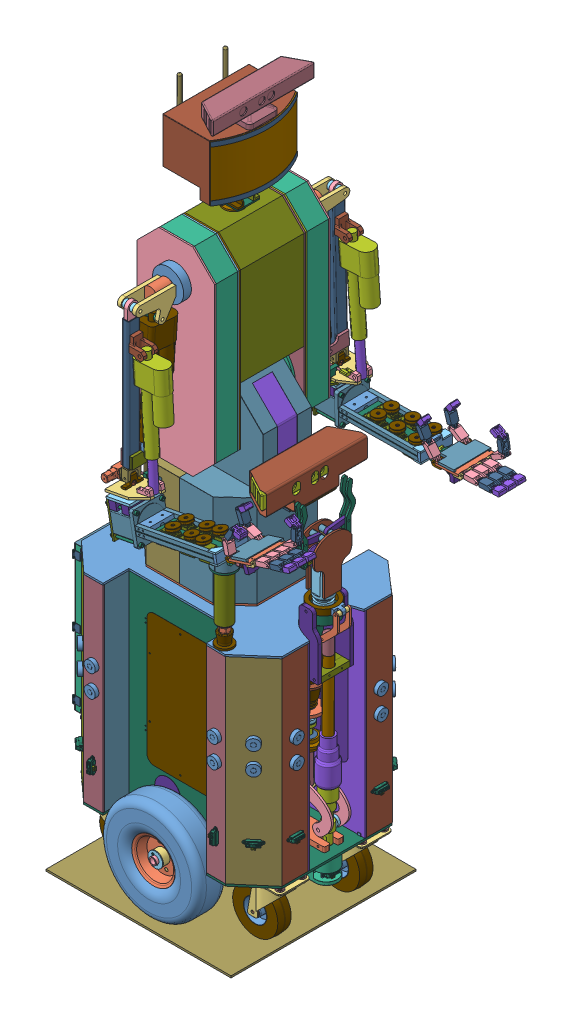
SolidWorks assembly sorbot, configuration По умолчанию. Lengths in mm. (continued)
Mates (geometry in assembly coordinates): (continued)
- Concentric42: concentric anti-aligned: cylinder of wall11-1 through (-271.9003 171.4368 -274.4564) axis (-1 0 0) radius 2; cylinder of computer.box.screw.fixture-4 through (-267.4772 171.4368 -274.4564) axis (1 0 0) radius 2
- Concentric43: concentric anti-aligned: cylinder of wall11-1 through (-271.9003 171.4368 0.207) axis (-1 0 0) radius 2; cylinder of computer.box.screw.fixture-3 through (-269.9003 171.4368 0.207) axis (1 0 0) radius 2
- Concentric44: concentric anti-aligned: cylinder of wall11-1 through (-271.9003 548.1505 0.207) axis (-1 0 0) radius 2; cylinder of computer.box.screw.fixture-2 through (-267.4772 548.1505 0.207) axis (1 0 0) radius 2
- Concentric45: concentric anti-aligned: cylinder of wall11-1 through (-271.9003 548.1505 -274.4564) axis (-1 0 0) radius 2; cylinder of computer.box.screw.fixture-1 through (-269.9003 548.1505 -274.4564) axis (1 0 0) radius 2
- Parallel10: parallel anti-aligned: plane of wall11-1 through (-271.9003 882.565 10.1667) normal (1 0 0); plane of us_sesnor_board-1 through (-254.9003 553.7811 -265.7072) normal (-1 0 0)
- Parallel11: parallel anti-aligned: plane of wall11-1 through (-271.9003 882.565 10.1667) normal (1 0 0); plane of us_sesnor_board-2 through (-254.9003 552.2966 -6.9008) normal (-1 0 0)
- Lock52: lock: unknown of wall11-1; unknown of wall-fixture-v2-1-2
- Lock54: lock: unknown of wall-fixture-v2-1-2; unknown of computer.box.screw.fixture-1
- Coincident100: coincident anti-aligned: plane of wall11-1 through (-271.9003 882.565 10.1667) normal (1 0 0); plane of wall-fixture-v2-1-1 through (-271.9003 624.2006 -10.7109) normal (-1 0 0)
- Lock55: lock: unknown of wall11-1; unknown of wall-fixture-v2-1-1
- Lock56: lock: unknown of wall-fixture-v2-1-1; unknown of computer.box.screw.fixture-2
- Coincident101: coincident: plane of us_sesnor_board-1 through (-261.9003 646.0902 -16.9266) normal (-1 0 0); plane of pillar.15mm-1 through (-261.9003 620.2581 -29.4638) normal (1 0 0)
- Coincident102: coincident: plane of us_sesnor_board-1 through (-261.9003 646.0902 -16.9266) normal (-1 0 0); plane of pillar.15mm-2 through (-261.9003 672.3698 -3.6565) normal (1 0 0)
- Coincident103: coincident: plane of us_sesnor_board-2 through (-278.4971 649.7829 -78.0769) normal (-1 0 0); plane of pillar.15mm-3 through (-278.4971 623.9508 -90.6141) normal (1 0 0)
- Coincident104: coincident: plane of us_sesnor_board-2 through (-278.4971 649.7829 -78.0769) normal (-1 0 0); plane of pillar.15mm-4 through (-278.4971 676.0625 -64.8068) normal (1 0 0)
- Concentric46: concentric anti-aligned: cylinder of us_sesnor_board-2 through (-278.4971 623.9508 -90.6141) axis (1 0 0) radius 1.5; cylinder of pillar.15mm-3 through (-278.4971 623.9508 -90.6141) axis (-1 0 0) radius 1.5
- Concentric47: concentric anti-aligned: cylinder of us_sesnor_board-2 through (-278.4971 676.0625 -64.8068) axis (1 0 0) radius 1.5; cylinder of pillar.15mm-4 through (-278.4971 676.0625 -64.8068) axis (-1 0 0) radius 1.5
- Concentric48: concentric anti-aligned: cylinder of us_sesnor_board-1 through (-261.9003 672.3698 -3.6565) axis (1 0 0) radius 1.5; cylinder of pillar.15mm-2 through (-261.9003 672.3698 -3.6565) axis (-1 0 0) radius 1.5
- Concentric49: concentric anti-aligned: cylinder of us_sesnor_board-1 through (-261.9003 620.2581 -29.4638) axis (1 0 0) radius 1.5; cylinder of pillar.15mm-1 through (-261.9003 620.2581 -29.4638) axis (-1 0 0) radius 1.5
- Lock57: lock: unknown of us_sesnor_board-2; unknown of pillar.15mm-3
- Lock58: lock: unknown of us_sesnor_board-2; unknown of pillar.15mm-4
- Lock59: lock: unknown of us_sesnor_board-1; unknown of pillar.15mm-1
- Lock60: lock: unknown of us_sesnor_board-1; unknown of pillar.15mm-2
- Coincident106: coincident anti-aligned: plane of wall-fixture-v2-1-2 through (-269.9003 624.1077 -280.8026) normal (1 0 0); plane of pillar.15mm-1 through (-269.9003 527.949 -278.2445) normal (-1 0 0)
- Coincident108: coincident anti-aligned: plane of wall-fixture-v2-1-1 through (-269.9003 624.2006 -10.7109) normal (1 0 0); plane of pillar.15mm-4 through (-269.9003 578.5762 6.3693) normal (-1 0 0)
- Coincident111: coincident: unknown of us_sesnor_board-3; unknown of pillar.10mm-5
- Coincident112: coincident: unknown of us_sesnor_board-3; unknown of pillar.10mm-6
- Concentric51: concentric anti-aligned: cylinder of us_sesnor_board-3 through (-93.4926 309.8196 -440.0551) axis (0 1 0) radius 1.5; cylinder of pillar.10mm-6 through (-93.4926 309.8196 -440.0551) axis (0 -1 0) radius 1.5
- Concentric52: concentric anti-aligned: cylinder of us_sesnor_board-3 through (-145.6043 309.8196 -414.2478) axis (0 1 0) radius 1.5; cylinder of pillar.10mm-5 through (-145.6043 309.8196 -414.2478) axis (0 -1 0) radius 1.5
- Coincident113: coincident: plane of us_sesnor_board-4 through (-60.2671 262.1055 -397.1446) normal (0 -1 0); plane of pillar.10mm-8 through (-34.435 262.1055 -409.6819) normal (0 1 0)
- Coincident114: coincident: plane of us_sesnor_board-4 through (-60.2671 262.1055 -397.1446) normal (0 -1 0); plane of pillar.10mm-7 through (-86.5467 262.1055 -383.8745) normal (0 1 0)
- Concentric53: concentric aligned: cylinder of us_sesnor_board-4 through (-86.5467 262.1055 -383.8745) axis (0 1 0) radius 1.5; circle of pillar.10mm-7
- Concentric54: concentric anti-aligned: cylinder of us_sesnor_board-4 through (-34.435 262.1055 -409.6819) axis (0 1 0) radius 1.5; cylinder of pillar.10mm-8 through (-34.435 262.1055 -409.6819) axis (0 -1 0) radius 1.5
- Lock61: lock: unknown of us_sesnor_board-3; unknown of pillar.10mm-5
- Lock62: lock: unknown of us_sesnor_board-3; unknown of pillar.10mm-6
- Lock63: lock: unknown of us_sesnor_board-4; unknown of pillar.10mm-7
- Lock64: lock: unknown of us_sesnor_board-4; unknown of pillar.10mm-8
- Coincident117: coincident anti-aligned: plane of wall7-v1-2 through (-197.4428 -52.2153 -351.9628) normal (0.67421 0 0.73854); plane of pillar.10mm-5 through (-235.454 251.2596 -317.2625) normal (-0.67421 0 -0.73854)
- Coincident118: coincident anti-aligned: plane of wall7-v1-1 through (-271.8817 -52.2153 10.1837) normal (0.67421 0 -0.73854); plane of pillar.10mm-7 through (-215.1295 251.2596 61.9925) normal (-0.67421 0 0.73854)
- Lock65: lock: unknown of bottom-2; unknown of wall7-v1-2
- Lock68: lock: unknown of bottom-2; unknown of wall-fixture-v1-2
- Parallel17: parallel anti-aligned: plane of wall-fixture-v2-1 through (-212.277 624.3178 64.5573) normal (-0.73854 -0.000294 -0.67421); unknown of DC-DC-12-24-1
- Parallel18: parallel anti-aligned: plane of wall7-v1-1 through (-271.8817 -52.2153 10.1837) normal (0.67421 0 -0.73854); unknown of DC-DC-12-24-1
- Coincident119: coincident anti-aligned: plane of wall7-v1-1 through (-271.8817 -52.2153 10.1837) normal (0.67421 0 -0.73854); line of DC-DC-12-24-fixture-1 through (-218.8855 352.3898 58.5637) axis (-0.67421 0 0.73854)
- Lock69: lock: unknown of wall7-v1-1; unknown of wall-fixture-v2-1
- Parallel20: parallel aligned: plane of wall-fixture-v2-1 through (-212.277 624.3178 64.5573) normal (-0.73854 -0.000294 -0.67421); unknown of DC-DC-12-24-fixture-1
- Coincident124: coincident anti-aligned: unknown of DC-DC-12-24-1; line of DC-DC-12-24-fixture-p1-1 through (-195.7071 367.4849 54.6738) axis (0.67421 0 -0.73854)
- Coincident125: coincident anti-aligned: unknown of DC-DC-12-24-fixture-1; line of DC-DC-12-24-fixture-p2-1 through (-197.3861 337.4849 56.5261) axis (-0.67421 0 0.73854)
- Coincident126: coincident aligned: unknown of DC-DC-12-24-fixture-p2-1; unknown of DC-DC-12-24-fixture-p1-1
- Coincident127: coincident aligned: unknown of DC-DC-12-24-fixture-p1-1; unknown of DC-DC-12-24-fixture-p2-1
- Coincident128: coincident anti-aligned: line of DC-DC-12-24-fixture-p1-1 through (-197.0555 367.4849 56.1509) axis (-0.67421 0 0.73854); unknown of DC-DC-12-24-fixture-p2-1
- Parallel21: parallel anti-aligned: unknown of DC-DC-12-24-fixture-1; unknown of DC-DC-12-24-fixture-p1-1
- Coincident129: coincident aligned: unknown of DC-DC-12-24-fixture-1; unknown of DC-DC-12-24-fixture-p2-1
- Coincident131: coincident anti-aligned: unknown of DC-DC-12-24-fixture-1; unknown of DC-DC-12-24-fixture-p1-1
- Coincident132: coincident anti-aligned: unknown of DC-DC-12-24-1; unknown of DC-DC-12-24-fixture-1
- Coincident133: coincident anti-aligned: plane of wall7-v1-1 through (-271.8817 -52.2153 10.1837) normal (0.67421 0 -0.73854); plane of DC-DC-12-24-fixture-2 through (-245.4729 352.3793 34.2921) normal (-0.67421 0 0.73854)
- Coincident134: coincident anti-aligned: unknown of DC-DC-12-24-1; unknown of DC-DC-12-24-fixture-2
- Coincident135: coincident aligned: unknown of DC-DC-12-24-fixture-1; unknown of DC-DC-12-24-fixture-2
- Lock73: lock: unknown of DC-DC-12-24-fixture-p1-1; unknown of DC-DC-12-24-fixture-p2-1
- Lock74: lock: unknown of DC-DC-12-24-fixture-p2-1; unknown of DC-DC-12-24-fixture-2
- Coincident136: coincident anti-aligned: plane of SD-25A-5-1 through (163.4873 75.504 -48.2424) normal (0 0 -1); plane of pillar.10mm-10 through (212.0094 150.4897 -48.2424) normal (0 0 1)
- Coincident137: coincident anti-aligned: plane of SD-25A-5-1 through (163.4873 75.504 -48.2424) normal (0 0 -1); plane of pillar.10mm-9 through (211.9932 95.4897 -48.2424) normal (0 0 1)
- Concentric55: concentric aligned: cylinder of SD-25A-5-1 through (212.0094 150.4897 -43.2424) axis (0 0 -1) radius 1.5; cylinder of pillar.10mm-10 through (212.0094 150.4897 -48.2424) axis (0 0 -1) radius 1.5
- Concentric56: concentric aligned: cylinder of SD-25A-5-1 through (211.9932 95.4897 -43.2424) axis (0 0 -1) radius 1.5; cylinder of pillar.10mm-9 through (211.9932 95.4897 -48.2424) axis (0 0 -1) radius 1.5
- Coincident138: coincident anti-aligned: plane of wall2-1 through (21.1889 831.1682 -58.2424) normal (0 0 1); plane of pillar.10mm-10 through (212.0094 150.4897 -58.2424) normal (0 0 -1)
- Coincident139: coincident anti-aligned: plane of wall-fixture-9-2 through (19.1889 577.5289 -196.2424) normal (-1 0 0); plane of platform.motor.drivers-1/dirvers.motor.assembly-1 through (19.1889 217.3926 -68.2424) normal (1 0 0)
- Lock75: lock: unknown of wall1-1; unknown of wall-fixture-9-2
- Distance39: distance = 5 mm aligned: plane of wall-fixture-9-2 through (19.1889 577.5289 -218.2424) normal (0 0 -1); plane of platform.motor.drivers-1/dirvers.motor.assembly-1 through (17.1889 222.3926 -213.2424) normal (0 0 -1)
- Coincident140: coincident anti-aligned: plane of wall10-1 through (-146.6756 864.7556 8.4522) normal (0 0 -1); plane of computer.box.screw.fixture-5 through (-89.5362 420.1505 8.4522) normal (0 0 1)
- Parallel22: parallel anti-aligned: plane of wall10-1 through (-84.5362 180.1505 8.4522) normal (0 1 0); plane of computer.box.screw.fixture-5 through (-84.5362 407.6505 -1.5478) normal (0 -1 0)
- Parallel24: parallel anti-aligned: plane of computer.box.screw.fixture-5 through (-84.5362 407.6505 -1.5478) normal (0 -1 0); plane of computer.box.screw.fixture-6 through (-94.5362 272.6505 -1.5478) normal (0 1 0)
- Coincident141: coincident anti-aligned: plane of wall10-1 through (-146.6756 864.7556 8.4522) normal (0 0 -1); plane of computer.box.screw.fixture-6 through (-89.5362 260.1505 8.4522) normal (0 0 1)
- Parallel25: parallel anti-aligned: plane of computer.box.screw.fixture-5 through (-84.5362 407.6505 -1.5478) normal (0 -1 0); plane of computer.box.screw.fixture-7 through (70.4638 432.6505 -1.5478) normal (0 1 0)
- Coincident142: coincident anti-aligned: plane of wall10-1 through (-146.6756 864.7556 8.4522) normal (0 0 -1); plane of computer.box.screw.fixture-7 through (75.4638 420.1505 8.4522) normal (0 0 1)
- Parallel26: parallel anti-aligned: plane of computer.box.screw.fixture-5 through (-84.5362 407.6505 -1.5478) normal (0 -1 0); plane of computer.box.screw.fixture-8 through (70.4638 272.6505 -1.5478) normal (0 1 0)
- Coincident143: coincident anti-aligned: plane of wall10-1 through (-146.6756 864.7556 8.4522) normal (0 0 -1); plane of computer.box.screw.fixture-8 through (75.4638 260.1505 8.4522) normal (0 0 1)
- Concentric57: concentric anti-aligned: cylinder of wall10-1 through (-89.5362 420.1505 8.4522) axis (0 0 1) radius 2; cylinder of computer.box.screw.fixture-5 through (-89.5362 420.1505 8.4522) axis (0 0 -1) radius 2
- Concentric58: concentric anti-aligned: cylinder of wall10-1 through (-89.5362 260.1505 8.4522) axis (0 0 1) radius 2; cylinder of computer.box.screw.fixture-6 through (-89.5362 260.1505 8.4522) axis (0 0 -1) radius 2
- Concentric59: concentric anti-aligned: cylinder of wall10-1 through (75.4638 420.1505 8.4522) axis (0 0 1) radius 2; cylinder of computer.box.screw.fixture-7 through (75.4638 420.1505 8.4522) axis (0 0 -1) radius 2
- Concentric60: concentric anti-aligned: cylinder of wall10-1 through (75.4638 260.1505 8.4522) axis (0 0 1) radius 2; cylinder of computer.box.screw.fixture-8 through (75.4638 260.1505 8.4522) axis (0 0 -1) radius 2
- Coincident144: coincident anti-aligned: plane of wall10-1 through (-146.6756 864.7556 8.4522) normal (0 0 -1); plane of computer.box.screw.fixture-10 through (-7.0362 505.1505 8.4522) normal (0 0 1)
- Coincident145: coincident anti-aligned: plane of wall10-1 through (-146.6756 864.7556 8.4522) normal (0 0 -1); plane of computer.box.screw.fixture-9 through (-7.0362 175.1505 8.4522) normal (0 0 1)
- Concentric61: concentric anti-aligned: cylinder of wall10-1 through (-7.0362 505.1505 8.4522) axis (0 0 1) radius 2; cylinder of computer.box.screw.fixture-10 through (-7.0362 505.1505 8.4522) axis (0 0 -1) radius 2
- Concentric62: concentric anti-aligned: cylinder of wall10-1 through (-7.0362 175.1505 8.4522) axis (0 0 1) radius 2; cylinder of computer.box.screw.fixture-9 through (-7.0362 175.1505 8.4522) axis (0 0 -1) radius 2
- Parallel27: parallel anti-aligned: plane of wall10-v1-1 through (-84.4656 180.1505 -290.2798) normal (0 1 0); plane of computer.box.screw.fixture-12 through (70.5344 407.6505 -276.2798) normal (0 -1 0)
- Coincident146: coincident anti-aligned: plane of wall10-v1-1 through (132.8227 864.7556 -286.2798) normal (0 0 1); plane of computer.box.screw.fixture-12 through (75.5344 420.1505 -286.2798) normal (0 0 -1)
- Parallel28: parallel anti-aligned: plane of computer.box.screw.fixture-16 through (-94.4656 432.6505 -276.2798) normal (0 1 0); plane of computer.box.screw.fixture-12 through (70.5344 407.6505 -276.2798) normal (0 -1 0)
- Parallel29: parallel anti-aligned: plane of computer.box.screw.fixture-12 through (70.5344 407.6505 -276.2798) normal (0 -1 0); plane of computer.box.screw.fixture-15 through (-94.4656 272.6505 -276.2798) normal (0 1 0)
- Parallel30: parallel anti-aligned: plane of computer.box.screw.fixture-12 through (70.5344 407.6505 -276.2798) normal (0 -1 0); plane of computer.box.screw.fixture-14 through (70.5344 272.6505 -276.2798) normal (0 1 0)
- Coincident147: coincident anti-aligned: plane of wall10-v1-1 through (132.8227 864.7556 -286.2798) normal (0 0 1); plane of computer.box.screw.fixture-16 through (-89.4656 420.1505 -286.2798) normal (0 0 -1)
- Coincident148: coincident anti-aligned: plane of wall10-v1-1 through (132.8227 864.7556 -286.2798) normal (0 0 1); plane of computer.box.screw.fixture-15 through (-89.4656 260.1505 -286.2798) normal (0 0 -1)
- Coincident149: coincident anti-aligned: plane of wall10-v1-1 through (132.8227 864.7556 -286.2798) normal (0 0 1); plane of computer.box.screw.fixture-14 through (75.5344 260.1505 -286.2798) normal (0 0 -1)
- Coincident150: coincident: plane of wall10-v1-1 through (132.8227 864.7556 -286.2798) normal (0 0 1); plane of computer.box.screw.fixture-13 through (-537.0801 640.6949 -286.2798) normal (0 0 -1)
- Concentric63: concentric anti-aligned: cylinder of wall10-v1-1 through (-89.4656 420.1505 -286.2798) axis (0 0 -1) radius 2; cylinder of computer.box.screw.fixture-16 through (-89.4656 420.1505 -286.2798) axis (0 0 1) radius 2
- Concentric64: concentric anti-aligned: cylinder of wall10-v1-1 through (-89.4656 260.1505 -286.2798) axis (0 0 -1) radius 2; cylinder of computer.box.screw.fixture-15 through (-89.4656 260.1505 -286.2798) axis (0 0 1) radius 2
- Concentric65: concentric anti-aligned: cylinder of wall10-v1-1 through (75.5344 420.1505 -286.2798) axis (0 0 -1) radius 2; cylinder of computer.box.screw.fixture-12 through (75.5344 420.1505 -286.2798) axis (0 0 1) radius 2
- Concentric66: concentric anti-aligned: cylinder of wall10-v1-1 through (75.5344 260.1505 -286.2798) axis (0 0 -1) radius 2; cylinder of computer.box.screw.fixture-14 through (75.5344 260.1505 -286.2798) axis (0 0 1) radius 2
- Parallel32: parallel: plane of wall10-v1-1 through (-84.4656 180.1505 -290.2798) normal (0 1 0); plane of computer.box.screw.fixture-13 through (-19.4656 500.1505 -276.2798) normal (0 -1 0)
- Coincident151: coincident: plane of wall10-v1-1 through (132.8227 864.7556 -286.2798) normal (0 0 1); plane of computer.box.screw.fixture-11 through (-6.9656 175.1505 -286.2798) normal (0 0 -1)
- Concentric67: concentric anti-aligned: cylinder of wall10-v1-1 through (-6.9656 505.1505 -286.2798) axis (0 0 -1) radius 2; cylinder of computer.box.screw.fixture-13 through (-6.9656 505.1505 -286.2798) axis (0 0 1) radius 2
- Concentric68: concentric anti-aligned: cylinder of wall10-v1-1 through (-6.9656 175.1505 -286.2798) axis (0 0 -1) radius 2; cylinder of computer.box.screw.fixture-11 through (-6.9656 175.1505 -286.2798) axis (0 0 1) radius 2
- Lock76: lock: unknown of wall10-1; unknown of computer.box.screw.fixture-5
- Lock77: lock: unknown of wall10-1; unknown of computer.box.screw.fixture-6
- Lock78: lock: unknown of wall10-1; unknown of computer.box.screw.fixture-9
- Lock79: lock: unknown of wall10-1; unknown of computer.box.screw.fixture-10
- Lock80: lock: unknown of wall10-1; unknown of computer.box.screw.fixture-7
- Lock81: lock: unknown of wall10-1; unknown of computer.box.screw.fixture-8
- Lock82: lock: unknown of wall10-v1-1; unknown of computer.box.screw.fixture-16
- Lock83: lock: unknown of wall10-v1-1; unknown of computer.box.screw.fixture-15
- Lock84: lock: unknown of wall10-v1-1; unknown of computer.box.screw.fixture-11
- Lock85: lock: unknown of wall10-v1-1; unknown of computer.box.screw.fixture-12
- Lock86: lock: unknown of wall10-v1-1; unknown of computer.box.screw.fixture-14
- Lock87: lock: unknown of wall10-v1-1; unknown of computer.box.screw.fixture-13
- Concentric69: concentric aligned: cylinder of wall10-1 through (-7.0362 505.1505 8.4522) axis (0 0 1) radius 2; cylinder of wall10-cap-1 through (-7.0362 505.1505 12.4522) axis (0 0 1) radius 2
- Concentric70: concentric aligned: cylinder of wall10-cap-2 through (-6.9656 505.1505 -286.6821) axis (0 0 1) radius 2; cylinder of computer.box.screw.fixture-13 through (-6.9656 505.1505 -282.1821) axis (0 0 1) radius 2
- Coincident152: coincident anti-aligned: plane of wall10-v1-1 through (132.8227 864.7556 -282.1821) normal (0 0 1); plane of plates.fixture-1 through (-109.2054 480.3702 -282.1821) normal (0 0 -1)
- Lock88: lock: unknown of bottom-2; unknown of wall10-v1-1
- Coincident153: coincident anti-aligned: plane of wall10-v1-1 through (132.8227 864.7556 -282.1821) normal (0 0 1); plane of plates.fixture-2 through (-109.2054 228.5986 -282.1821) normal (0 0 -1)
- Coincident154: coincident aligned: plane of plates.fixture-1 through (-109.2054 480.3702 -281.1821) normal (-1 0 0); plane of plates.fixture-2 through (-109.2054 228.5986 -281.1821) normal (-1 0 0)
- Lock89: lock: unknown of wall10-v1-1; unknown of plates.fixture-1
- Lock90: lock: unknown of wall10-v1-1; unknown of plates.fixture-2
- Coincident155: coincident anti-aligned: plane of left.plate-1 through (-11.6361 340.1505 -241.559) normal (0 0 -1); plane of plates.fixture-3 through (-81.9634 476.3702 -241.559) normal (0 0 1)
- Coincident156: coincident anti-aligned: plane of left.plate-1 through (-11.6361 340.1505 -241.559) normal (0 0 -1); plane of plates.fixture-4 through (-81.9634 224.5986 -241.559) normal (0 0 1)
- Parallel34: parallel anti-aligned: plane of wall10-v1-1 through (-84.4656 500.1505 -286.1821) normal (0 -1 0); plane of plates.fixture-3 through (-81.9634 477.3702 -242.559) normal (0 1 0)
- Parallel35: parallel anti-aligned: plane of wall10-v1-1 through (-84.4656 500.1505 -286.1821) normal (0 -1 0); plane of plates.fixture-4 through (-81.9634 225.5986 -242.559) normal (0 1 0)
- Concentric71: concentric anti-aligned: cylinder of plates.fixture-1 through (-101.7054 479.3702 -270.1821) axis (0 1 0) radius 2; cylinder of plate.console-1 through (-101.7054 479.3702 -270.1821) axis (0 -1 0) radius 2
- Coincident157: coincident anti-aligned: plane of plates.fixture-1 through (-109.2054 479.3702 -281.1821) normal (0 -1 0); plane of plate.console-1 through (-101.0285 479.3702 -253.0691) normal (0 1 0)
- Coincident158: coincident anti-aligned: plane of plates.fixture-3 through (-81.9634 477.3702 -242.559) normal (0 1 0); plane of plate.console-1 through (-101.0285 477.3702 -253.0691) normal (0 -1 0)
- Concentric72: concentric aligned: cylinder of plates.fixture-3 through (-74.4634 477.3702 -253.559) axis (0 -1 0) radius 2; cylinder of plate.console-1 through (-74.4634 479.3702 -253.559) axis (0 -1 0) radius 2
- Coincident159: coincident anti-aligned: plane of plates.fixture-2 through (-109.2054 227.5986 -281.1821) normal (0 -1 0); plane of plate.console-2 through (-101.0285 227.5986 -253.0691) normal (0 1 0)
- Concentric73: concentric anti-aligned: cylinder of plates.fixture-2 through (-101.7054 227.5986 -270.1821) axis (0 1 0) radius 2; cylinder of plate.console-2 through (-101.7054 227.5986 -270.1821) axis (0 -1 0) radius 2
- Concentric74: concentric aligned: cylinder of plates.fixture-4 through (-74.4634 225.5986 -253.559) axis (0 -1 0) radius 2; cylinder of plate.console-2 through (-74.4634 227.5986 -253.559) axis (0 -1 0) radius 2
- Coincident161: coincident anti-aligned: plane of plates.fixture-4 through (-81.9634 225.5986 -242.559) normal (0 1 0); plane of plate.console-2 through (-101.0285 225.5986 -253.0691) normal (0 -1 0)
- Coincident162: coincident aligned: plane of plates.fixture-3 through (-66.9634 476.3702 -242.559) normal (1 0 0); plane of plates.fixture-4 through (-66.9634 224.5986 -242.559) normal (1 0 0)
- Lock91: lock: unknown of left.plate-1; unknown of plates.fixture-3
- Lock92: lock: unknown of left.plate-1; unknown of plates.fixture-4
- Parallel33: parallel anti-aligned: plane of wall10-v1-1 through (132.8227 864.7556 -286.1821) normal (0 0 -1); plane of left.plate-1 through (-11.6361 340.1505 -239.559) normal (0 0 1)
- Concentric75: concentric anti-aligned: cylinder of left.plate-1 through (-74.4634 460.95 -239.559) axis (0 0 -1) radius 1.5; cylinder of plates.fixture-3 through (-74.4634 460.95 -260.5433) axis (0 0 1) radius 1.5
- Concentric76: concentric anti-aligned: cylinder of left.plate-1 through (-74.4634 209.1784 -239.559) axis (0 0 -1) radius 1.5; cylinder of plates.fixture-4 through (-74.4634 209.1784 -260.5433) axis (0 0 1) radius 1.5
- Concentric77: concentric aligned: cylinder of wall10-1 through (-101.7054 495.7903 8.4522) axis (0 0 1) radius 1.5; cylinder of plates.fixture-5 through (-101.7054 495.7903 -10.5321) axis (0 0 1) radius 1.5
- Coincident164: coincident anti-aligned: plane of wall10-1 through (-146.6756 864.7556 8.4522) normal (0 0 -1); plane of plates.fixture-5 through (-94.2054 480.3702 8.4522) normal (0 0 1)
- Coincident165: coincident anti-aligned: plane of wall10-1 through (-146.6756 864.7556 8.4522) normal (0 0 -1); plane of plates.fixture-6 through (-94.2054 228.5986 8.4522) normal (0 0 1)
- Concentric78: concentric aligned: cylinder of wall10-1 through (-101.7054 244.0187 8.4522) axis (0 0 1) radius 1.5; cylinder of plates.fixture-6 through (-101.7054 244.0187 -10.5321) axis (0 0 1) radius 1.5
- Concentric79: concentric aligned: cylinder of plates.fixture-5 through (-101.7054 479.3702 -3.5478) axis (0 1 0) radius 2; cylinder of plate.console-3 through (-101.7054 477.3702 -3.5478) axis (0 1 0) radius 2
- Coincident166: coincident anti-aligned: plane of plates.fixture-5 through (-94.2054 479.3702 7.4522) normal (0 -1 0); plane of plate.console-3 through (-98.2147 479.3702 -20.3146) normal (0 1 0)
- Concentric80: concentric aligned: cylinder of plates.fixture-6 through (-101.7054 227.5986 -3.5478) axis (0 1 0) radius 2; cylinder of plate.console-4 through (-101.7054 225.5986 -3.5478) axis (0 1 0) radius 2
- Coincident167: coincident anti-aligned: plane of plates.fixture-6 through (-94.2054 227.5986 7.4522) normal (0 -1 0); plane of plate.console-4 through (-98.2147 227.5986 -20.3146) normal (0 1 0)
- Coincident168: coincident anti-aligned: unknown of right.plate-1; unknown of plates.fixture-7
- Coincident169: coincident anti-aligned: unknown of right.plate-1; unknown of plates.fixture-8
- Concentric86: concentric anti-aligned: cylinder of right.plate-1 through (-71.7547 460.95 -9.5043) axis (0 0 1) radius 1.5; cylinder of plates.fixture-7 through (-71.7547 460.95 12.48) axis (0 0 -1) radius 1.5
- Concentric87: concentric anti-aligned: cylinder of right.plate-1 through (-71.7547 471.1225 -9.5043) axis (0 0 1) radius 1.5; cylinder of plates.fixture-7 through (-71.7547 471.1225 12.48) axis (0 0 -1) radius 1.5
- Coincident171: coincident anti-aligned: plane of plate.console-3 through (-98.2147 477.3702 -20.3146) normal (0 -1 0); plane of plates.fixture-7 through (-64.5944 477.3702 -26.4493) normal (0 1 0)
- Concentric88: concentric anti-aligned: cylinder of right.plate-1 through (-71.7547 209.1784 -9.5043) axis (0 0 1) radius 1.5; cylinder of plates.fixture-8 through (-71.7547 209.1784 12.48) axis (0 0 -1) radius 1.5
- Concentric89: concentric anti-aligned: cylinder of right.plate-1 through (-71.7547 219.3509 -9.5043) axis (0 0 1) radius 1.5; cylinder of plates.fixture-8 through (-71.7547 219.3509 12.48) axis (0 0 -1) radius 1.5
- Coincident172: coincident anti-aligned: plane of plate.console-4 through (-98.2147 225.5986 -20.3146) normal (0 -1 0); plane of plates.fixture-8 through (-64.5944 225.5986 -26.4493) normal (0 1 0)
- Lock93: lock: unknown of right.plate-1; unknown of plates.fixture-7
- Lock94: lock: unknown of right.plate-1; unknown of plates.fixture-8
- Parallel36: parallel anti-aligned: plane of wall10-1 through (-146.6756 864.7556 8.4522) normal (0 0 -1); plane of right.plate-1 through (-9.2671 340.1505 -27.4493) normal (0 0 1)
- Concentric90: concentric anti-aligned: cylinder of plate.console-3 through (-72.0944 477.3702 -15.4493) axis (0 1 0) radius 2; cylinder of plates.fixture-7 through (-72.0944 477.3702 -15.4493) axis (0 -1 0) radius 2
- Concentric91: concentric anti-aligned: cylinder of plate.console-4 through (-72.0944 225.5986 -15.4493) axis (0 1 0) radius 2; cylinder of plates.fixture-8 through (-72.0944 225.5986 -15.4493) axis (0 -1 0) radius 2
- Lock95: lock: unknown of bottom-2; unknown of wall10-1
- Coincident174: coincident aligned: plane of bottom-2 through (74.7083 51.9368 -286.1821) normal (0 0 -1); plane of wall10-v1-1 through (132.8227 864.7556 -286.1821) normal (0 0 -1)
- Lock96: lock: unknown of bottom-2; unknown of wall9-4
- Lock97: lock: unknown of bottom-2; unknown of wall8-2
- Lock98: lock: unknown of bottom-2; unknown of wall7-3
- Lock99: lock: unknown of bottom-2; unknown of wall6-3
- Lock100: lock: unknown of bottom-2; unknown of wall6-1
- Lock101: lock: unknown of bottom-2; unknown of wall7-1
- Lock102: lock: unknown of bottom-2; unknown of wall8-1
- Lock103: lock: unknown of bottom-2; unknown of wall9-1
- Lock104: lock: unknown of wall9-4; unknown of wall-fixture-v1-5
- Lock105: lock: unknown of wall8-2; unknown of wall-fixture-v1-6
- Lock106: lock: unknown of wall8-2; unknown of wall-fixture-v2-2-1
- Lock107: lock: unknown of wall7-3; unknown of wall-fixture-v2-3-1
- Lock108: lock: unknown of wall6-3; unknown of wall-fixture-v1-7
- Lock109: lock: unknown of wall6-1; unknown of wall-fixture-v1-8
- Lock110: lock: unknown of wall6-1; unknown of wall-fixture-v2-4-1
- Lock111: lock: unknown of wall7-1; unknown of wall-fixture-v2-5-1
- Lock112: lock: unknown of wall8-1; unknown of wall-fixture-v1-9
- Lock113: lock: unknown of wall9-1; unknown of wall-fixture-v1-10
- Coincident175: coincident: line of us_sesnor_board-10 through (749.4268 107.2544 211.7829) axis (0 -1 0); unknown of pillar.10mm-22
- Concentric92: concentric anti-aligned: cylinder of us_sesnor_board-10 through (775.2589 107.2544 199.2456) axis (0 1 0) radius 1.5; cylinder of pillar.10mm-22 through (775.2589 107.2544 199.2456) axis (0 -1 0) radius 1.5
- Coincident176: coincident: line of us_sesnor_board-10 through (749.4268 107.2544 211.7829) axis (0 -1 0); unknown of pillar.10mm-21
- Concentric93: concentric anti-aligned: cylinder of us_sesnor_board-10 through (723.1472 107.2544 225.053) axis (0 1 0) radius 1.5; cylinder of pillar.10mm-21 through (723.1472 107.2544 225.053) axis (0 -1 0) radius 1.5
- Coincident177: coincident: unknown of us_sesnor_board-9; unknown of pillar.10mm-20
- Concentric94: concentric anti-aligned: cylinder of us_sesnor_board-9 through (712.8236 123.0685 161.9115) axis (0 1 0) radius 1.5; cylinder of pillar.10mm-20 through (712.8236 123.0685 161.9115) axis (0 -1 0) radius 1.5
- Coincident178: coincident: unknown of us_sesnor_board-9; unknown of pillar.10mm-19
- Concentric95: concentric anti-aligned: cylinder of us_sesnor_board-9 through (660.7119 123.0685 187.7188) axis (0 1 0) radius 1.5; cylinder of pillar.10mm-19 through (660.7119 123.0685 187.7188) axis (0 -1 0) radius 1.5
- Coincident179: coincident: unknown of us_sesnor_board-8; unknown of pillar.10mm-18
- Concentric96: concentric anti-aligned: cylinder of us_sesnor_board-8 through (596.7218 144.8853 146.6678) axis (0 1 0) radius 1.5; cylinder of pillar.10mm-18 through (596.7218 144.8853 146.6678) axis (0 -1 0) radius 1.5
- Coincident180: coincident: unknown of us_sesnor_board-8; unknown of pillar.10mm-17
- Concentric97: concentric anti-aligned: cylinder of us_sesnor_board-8 through (648.8335 144.8853 120.8605) axis (0 1 0) radius 1.5; cylinder of pillar.10mm-17 through (648.8335 144.8853 120.8605) axis (0 -1 0) radius 1.5
- Coincident181: coincident: unknown of us_sesnor_board-7; unknown of pillar.10mm-16
- Concentric98: concentric anti-aligned: cylinder of us_sesnor_board-7 through (593.7432 170.0579 82.3435) axis (0 1 0) radius 1.5; cylinder of pillar.10mm-16 through (593.7432 170.0579 82.3435) axis (0 -1 0) radius 1.5
- Coincident182: coincident: unknown of us_sesnor_board-7; unknown of pillar.10mm-15
- Concentric99: concentric anti-aligned: cylinder of us_sesnor_board-7 through (541.6315 170.0579 108.1508) axis (0 1 0) radius 1.5; cylinder of pillar.10mm-15 through (541.6315 170.0579 108.1508) axis (0 -1 0) radius 1.5
- Coincident183: coincident: unknown of us_sesnor_board-6; unknown of pillar.10mm-14
- Coincident184: coincident: unknown of us_sesnor_board-6; unknown of pillar.10mm-13
- Concentric100: concentric anti-aligned: cylinder of us_sesnor_board-6 through (504.7031 219.2793 99.3663) axis (0 1 0) radius 1.5; cylinder of pillar.10mm-14 through (504.7031 219.2793 99.3663) axis (0 -1 0) radius 1.5
- Concentric101: concentric anti-aligned: cylinder of us_sesnor_board-6 through (452.5914 219.2793 125.1736) axis (0 1 0) radius 1.5; cylinder of pillar.10mm-13 through (452.5914 219.2793 125.1736) axis (0 -1 0) radius 1.5
- Coincident185: coincident: unknown of us_sesnor_board-5; line of pillar.10mm-12 through (462.1177 251.3904 79.2617) axis (0 1 0)
- Coincident186: coincident: unknown of us_sesnor_board-5; line of pillar.10mm-11 through (410.006 251.3904 105.069) axis (0 1 0)
- Concentric102: concentric anti-aligned: cylinder of us_sesnor_board-5 through (462.1177 251.3904 79.2617) axis (0 1 0) radius 1.5; cylinder of pillar.10mm-12 through (462.1177 251.3904 79.2617) axis (0 -1 0) radius 1.5
- Concentric103: concentric anti-aligned: cylinder of us_sesnor_board-5 through (410.006 251.3904 105.069) axis (0 1 0) radius 1.5; cylinder of pillar.10mm-11 through (410.006 251.3904 105.069) axis (0 -1 0) radius 1.5
- Lock114: lock: unknown of us_sesnor_board-5; unknown of pillar.10mm-11
- Lock115: lock: unknown of us_sesnor_board-5; unknown of pillar.10mm-12
- Lock116: lock: unknown of us_sesnor_board-6; unknown of pillar.10mm-13
- Lock117: lock: unknown of us_sesnor_board-6; unknown of pillar.10mm-14
- Lock118: lock: unknown of us_sesnor_board-7; unknown of pillar.10mm-15
- Lock119: lock: unknown of us_sesnor_board-7; unknown of pillar.10mm-16
- Lock120: lock: unknown of us_sesnor_board-8; unknown of pillar.10mm-18
- Lock121: lock: unknown of us_sesnor_board-8; unknown of pillar.10mm-17
- Lock122: lock: unknown of us_sesnor_board-9; unknown of pillar.10mm-19
- Lock123: lock: unknown of us_sesnor_board-9; unknown of pillar.10mm-20
- Lock124: lock: unknown of us_sesnor_board-10; unknown of pillar.10mm-21
- Lock125: lock: unknown of us_sesnor_board-10; unknown of pillar.10mm-22
- Coincident187: coincident anti-aligned: plane of wall-fixture-v1-6 through (158.7521 559.4368 -350.1821) normal (0 0 1); plane of pillar.10mm-11 through (143.5283 296.7164 -350.1821) normal (0 0 -1)
- Parallel37: parallel anti-aligned: plane of wall8-2 through (132.798 585.1368 -356.1821) normal (0 1 0); plane of us_sesnor_board-5 through (172.7984 453.6148 -338.6821) normal (0 -1 0)
- Coincident188: coincident anti-aligned: plane of wall7-3 through (183.3311 693.5591 -352.2595) normal (-0.650583 0 0.759435); plane of pillar.10mm-13 through (225.1561 204.1572 -316.4293) normal (0.650583 0 -0.759435)
- Parallel38: parallel aligned: plane of wall7-3 through (98.7066 585.1505 -215.5106) normal (0 1 0); plane of us_sesnor_board-6 through (195.4456 258.9368 -326.7385) normal (0 1 0)
- Coincident190: coincident anti-aligned: plane of wall-fixture-v2-3-1 through (261.2073 551.4368 -262.8797) normal (-0.999998 0 0.00186); plane of pillar.10mm-15 through (261.2571 184.1572 -236.1088) normal (0.999998 0 -0.00186)
- Parallel40: parallel aligned: plane of wall6-1 through (141.4136 585.1505 -94.8266) normal (0 1 0); plane of wall6-3 through (141.4135 585.1505 -322.8954) normal (0 1 0)
- Coincident191: coincident anti-aligned: plane of wall-fixture-v1-8 through (261.1742 559.4368 -36.2424) normal (-1 0 0); plane of pillar.10mm-18 through (261.1742 184.1572 -8.9716) normal (1 0 0)
- Parallel41: parallel aligned: plane of wall6-1 through (141.4136 585.1505 -94.8266) normal (0 1 0); plane of us_sesnor_board-8 through (249.6742 537.5614 -38.2417) normal (0 1 0)
- Coincident192: coincident anti-aligned: plane of wall7-1 through (263.5537 693.5591 9.7838) normal (-0.650583 0 -0.759435); plane of pillar.10mm-19 through (202.949 204.1572 61.7019) normal (0.650583 0 0.759435)
- Parallel42: parallel aligned: plane of wall7-1 through (141.4136 585.1505 -94.8266) normal (0 1 0); plane of us_sesnor_board-9 through (217.6961 258.9368 33.9258) normal (0 1 0)
- Coincident193: coincident anti-aligned: plane of wall-fixture-v2-5-1 through (179.4039 91.4368 76.4522) normal (0 0 -1); plane of pillar.10mm-21 through (173.0129 296.7164 76.4522) normal (0 0 1)
- Parallel43: parallel anti-aligned: plane of wall8-1 through (184.8921 585.1368 82.4377) normal (0 1 0); plane of us_sesnor_board-10 through (143.7428 449.9398 64.9522) normal (0 -1 0)
- Distance40: distance = 190 mm aligned: plane of wall8-2 through (132.798 51.9368 -356.1821) normal (0 -1 0); plane of us_sesnor_board-5 through (172.7984 241.9368 -338.6821) normal (0 -1 0)
- Distance41: distance = 150 mm aligned: plane of us_sesnor_board-6 through (195.4456 201.9368 -326.7385) normal (0 -1 0); plane of wall7-3 through (183.3311 51.9368 -352.2595) normal (0 -1 0)
- Distance42: distance = 130 mm aligned: plane of us_sesnor_board-7 through (249.7027 181.9368 -265.3575) normal (0 -1 0); plane of wall6-3 through (263.1741 51.9368 -286.3112) normal (0 -1 0)
- Distance43: distance = 130 mm aligned: plane of us_sesnor_board-8 through (249.6742 181.9368 -38.2417) normal (0 -1 0); plane of wall6-1 through (263.1742 51.9368 -58.2424) normal (0 -1 0)
- Distance44: distance = 150 mm aligned: plane of us_sesnor_board-9 through (217.6961 201.9368 33.9258) normal (0 -1 0); plane of wall7-1 through (263.5537 51.9368 9.7838) normal (0 -1 0)
- Distance45: distance = 190 mm aligned: plane of us_sesnor_board-10 through (143.7428 241.9368 64.9522) normal (0 -1 0); plane of wall8-1 through (184.8921 51.9368 82.4377) normal (0 -1 0)
- Lock126: lock: unknown of wall8-2; unknown of us_sesnor_board-5
- Lock127: lock: unknown of wall7-3; unknown of us_sesnor_board-6
- Lock130: lock: unknown of wall7-1; unknown of us_sesnor_board-9
- Lock131: lock: unknown of wall8-1; unknown of us_sesnor_board-10
- Lock132: lock: unknown of acdc.220V.filter-1; unknown of pillar.10mm-23
- Lock133: lock: unknown of acdc.220V.filter-1; unknown of pillar.10mm-24
- Parallel45: parallel anti-aligned: plane of wall7-3 through (183.3311 693.5591 -352.2595) normal (-0.650583 0 0.759435); unknown of acdc.12v.power.supply-1
- Parallel46: parallel aligned: line of wall7-3 through (263.6412 585.1505 -283.4604) axis (0 -1 0); line of acdc.12v.power.supply-1 through (309.2456 375.1425 -124.6018) axis (0 -1 0)
- Coincident197: coincident anti-aligned: unknown of acdc.12v.power.supply-1; unknown of AC-DC-12-fixture-2
- Coincident198: coincident: line of acdc.12v.power.supply-1 through (271.2738 255.1356 -157.131) axis (0 1 0); unknown of AC-DC-12-fixture-2
- Coincident199: coincident anti-aligned: unknown of acdc.12v.power.supply-1; unknown of AC-DC-12-fixture-1
- Coincident201: coincident: line of acdc.12v.power.supply-1 through (309.2456 375.1425 -124.6018) axis (0 -1 0); line of AC-DC-12-fixture-1 through (329.4137 316.6958 -148.1443) axis (-0.759435 0 -0.650583)
- Coincident202: coincident aligned: plane of AC-DC-12-fixture-1 through (185.5021 169.4229 -342.8791) normal (0 1 0); plane of AC-DC-12-fixture-2 through (185.5021 169.4229 -316.3791) normal (0 1 0)
- Lock134: lock: unknown of acdc.12v.power.supply-1; unknown of AC-DC-12-fixture-1
- Lock135: lock: unknown of acdc.12v.power.supply-1; unknown of AC-DC-12-fixture-2
- Lock137: lock: unknown of DC-DC-12-24-1; unknown of DC-DC-12-24-fixture-2
- Lock138: lock: unknown of DC-DC-12-24-1; unknown of DC-DC-12-24-fixture-1
- Coincident208: coincident anti-aligned: plane of wall-fixture-v1-6 through (138.7521 559.4368 -350.1821) normal (1 0 0); plane of AC-DC-12-fixture-1 through (138.7521 154.3322 -328.3791) normal (-1 0 0)
- Coincident209: coincident anti-aligned: plane of wheel.disk-1 through (-6.6918 11.9368 -256.3681) normal (0 0 1); plane of encoder-2-1 through (-6.6918 11.9368 -256.3681) normal (0 0 -1)
- Coincident210: coincident anti-aligned: plane of wheel.disk-2 through (-6.6918 11.9368 -15.8681) normal (0 0 -1); plane of encoder-2-2 through (-6.6918 11.9368 -15.8681) normal (0 0 1)
- Concentric105: concentric aligned: cylinder of wheel.stop.bearing-2/wheel.stop.bearing.p1-1 through (-6.6918 11.9368 -252.3681) axis (0 0 -1) radius 20; cylinder of encoder-2-1 through (-6.6918 11.9368 -255.8681) axis (0 0 -1) radius 20.05
- Concentric106: concentric anti-aligned: cylinder of wheel.stop.bearing-3/wheel.stop.bearing.p1-2 through (-6.6918 11.9368 -19.8681) axis (0 0 1) radius 20; cylinder of encoder-2-2 through (-6.6918 11.9368 -15.8681) axis (0 0 -1) radius 20.05
- Coincident211: coincident anti-aligned: plane of wall-fixture-v1-8 through (261.1742 559.4368 -56.2424) normal (0 0 1); plane of pillar.10mm-23 through (235.8821 551.7681 -56.2424) normal (0 0 -1)
- Coincident212: coincident anti-aligned: plane of wall7-3 through (183.3311 693.5591 -352.2595) normal (-0.650583 0 0.759435); plane of pillar.10mm-1 through (199.1381 516.894 -338.7181) normal (0.650583 0 -0.759435)
- Coincident213: coincident anti-aligned: plane of wall10-1 through (-146.6756 864.7556 8.4522) normal (0 0 -1); plane of DC-DC-12-24-fixture-2 through (-7.0001 536.9758 8.4522) normal (0 0 1)
- Parallel47: parallel aligned: plane of bottom-2 through (-49.3372 51.9368 -286.1821) normal (0 1 0); plane of DC-DC-12-24-1 through (-62.5405 587.4758 -10.0478) normal (0 1 0)
- Coincident214: coincident anti-aligned: plane of wall-fixture-v1-10 through (138.9009 584.9368 6.4522) normal (1 0 0); plane of spool.220v-1/spool.ac220v.base-1 through (138.9009 432.1505 27.9371) normal (-1 0 0)
- Coincident215: coincident anti-aligned: plane of wall-fixture-v1-9 through (138.9009 559.4368 76.4522) normal (0 0 -1); plane of spool.220v-1/spool.ac220v.base-1 through (143.9009 497.1505 76.4522) normal (0 0 1)
- Distance46: distance = 88 mm aligned: plane of wall9-1 through (141.4136 585.1505 -94.8266) normal (0 1 0); plane of spool.220v-1/spool.ac220v.base-1 through (143.9009 497.1505 76.4522) normal (0 1 0)
- Coincident216: coincident anti-aligned: plane of wall2-2 through (21.1889 831.1682 -212.2424) normal (0 0 1); plane of wall2.cap-1 through (201.6115 220.4739 -212.2424) normal (0 0 -1)
- Coincident217: coincident anti-aligned: plane of wall2-1 through (21.1889 831.1682 -62.2424) normal (0 0 -1); plane of wall2.cap-2 through (201.1134 530.6582 -62.2424) normal (0 0 1)
- Coincident218: coincident anti-aligned: plane of cap-1 through (216.6678 590.1505 -83.5666) normal (0 1 0); plane of spool.220v.inlet-1 through (160.9714 590.1505 61.3093) normal (0 -1 0)
- Concentric107: concentric anti-aligned: cylinder of cap-1 through (160.9714 585.1505 61.3093) axis (0 1 0) radius 8; cylinder of spool.220v.inlet-1 through (160.9714 595.1505 61.3093) axis (0 -1 0) radius 8
- Concentric108: concentric aligned: cylinder of spool.220v.inlet-1 through (160.9714 595.1505 61.3093) axis (0 -1 0) radius 22; cylinder of charger.module-1/charger.module.handle-1 through (160.9714 772.2706 61.3093) axis (0 -1 0) radius 20
- Parallel48: parallel anti-aligned: plane of bottom-2 through (267.1742 51.9368 -285.7013) normal (1 0 0); plane of scanning.distance.meter.platform.bottom-1/scanning.distance.meter.case-1 through (212.6113 -13.9132 -136.8636) normal (-1 0 0)
- Distance47: distance = 140.685 mm: plane of scanning.distance.meter.platform.bottom-1/servo.sm-s3317s-1 through (251.6524 18.4368 -128.7136) normal (0 0 1); line of bottom-2 through (267.1742 51.9368 11.9714) axis (0 -1 0)
- Coincident219: coincident anti-aligned: plane of bottom-2 through (-49.3372 46.4368 -286.1821) normal (0 -1 0); plane of scanning.distance.meter.platform.bottom-1/servo.sm-s3317s-1 through (236.0024 46.4368 -136.8636) normal (0 1 0)
- Coincident220: coincident anti-aligned: plane of body.cover-1 through (132.0303 1000.7397 -71.9555) normal (-1 0 0); plane of body.cover.glass-1 through (132.0303 942.6564 -137.0438) normal (1 0 0)
- Distance49: distance = 13 mm: line of body.cover-1 through (132.0303 930.9934 -163.9555) axis (0 1 0); plane of body.cover.glass-1 through (132.0303 999.4971 -176.9555) normal (0 0 -1)
- Lock139: lock: unknown of turret.table-1; unknown of body.cover-1
- Coincident221: coincident anti-aligned: plane of body.cover-1 through (132.5303 1000.7397 -71.9555) normal (1 0 0); plane of frontal.kinect.plate-1 through (132.5303 856.8423 -76.6669) normal (-1 0 0)
- Parallel49: parallel aligned: plane of body.cover-1 through (132.5303 1000.7397 -71.9555) normal (1 0 0); plane of kinect-1 through (204.8758 870.3423 -166.6669) normal (1 0 0)
- Coincident224: coincident anti-aligned: plane of kinect-1 through (149.8758 857.3423 -166.6669) normal (0 -1 0); plane of frontal.kinect.cover-1 through (172.5303 857.3423 -136.6669) normal (0 1 0)
- Distance51: distance = 20 mm aligned: plane of kinect-1 through (149.8758 870.3423 -176.6669) normal (0 0 -1); plane of frontal.kinect.plate-1 through (132.5303 856.8423 -196.6669) normal (0 0 -1)
- Coincident226: coincident anti-aligned: plane of body.cover-1 through (132.5303 1000.7397 -71.9555) normal (1 0 0); plane of frontal.kinect.plate.fixture-1 through (132.5303 854.8423 -96.6669) normal (-1 0 0)
- Coincident227: coincident anti-aligned: plane of body.cover-1 through (132.5303 1000.7397 -71.9555) normal (1 0 0); plane of frontal.kinect.plate.fixture-2 through (132.5303 854.8423 -196.6669) normal (-1 0 0)
- Coincident228: coincident anti-aligned: plane of frontal.kinect.plate-1 through (172.5303 854.8423 -136.6669) normal (0 -1 0); plane of frontal.kinect.plate.fixture-1 through (134.0303 854.8423 -76.6669) normal (0 1 0)
- Coincident229: coincident anti-aligned: plane of frontal.kinect.plate-1 through (172.5303 854.8423 -136.6669) normal (0 -1 0); plane of frontal.kinect.plate.fixture-2 through (134.0303 854.8423 -176.6669) normal (0 1 0)
- Coincident230: coincident aligned: plane of frontal.kinect.plate-1 through (132.5303 856.8423 -76.6669) normal (0 0 1); plane of frontal.kinect.plate.fixture-1 through (134.0303 854.8423 -76.6669) normal (0 0 1)
- Coincident231: coincident aligned: plane of frontal.kinect.plate-1 through (132.5303 856.8423 -196.6669) normal (0 0 -1); plane of frontal.kinect.plate.fixture-2 through (134.0303 854.8423 -196.6669) normal (0 0 -1)
- Coincident232: coincident anti-aligned: plane of body.cover-1 through (49.9766 1082.7934 -71.9555) normal (-0.707107 -0.707107 0); plane of body.cover.glass-1 through (159.572 973.1981 -137.0438) normal (0.707107 0.707107 0)
- Coincident234: coincident anti-aligned: plane of frontal.kinect.plate-1 through (172.5303 856.8423 -136.6669) normal (0 1 0); plane of frontal.kinect.cover-1 through (172.5303 856.8423 -136.6669) normal (0 -1 0)
- Lock140: lock: unknown of turret.table-1; unknown of body.cover.back-1
- Coincident238: coincident anti-aligned: plane of body.cover.back-1 through (-90.4598 1083.147 -201.9735) normal (-0.707107 0.707107 0); plane of back.camera.housing-1 through (-157.6642 1015.9425 -137.3735) normal (0.707107 -0.707107 0)
- Parallel50: parallel anti-aligned: plane of body.cover.back-1 through (-172.1599 861.5934 -71.3735) normal (0 0 1); plane of back.camera.housing-1 through (-143.5221 1030.0847 -182.3735) normal (0 0 -1)
- Distance52: distance = 21 mm aligned: plane of back.camera.housing-1 through (-143.5221 1030.0847 -92.3735) normal (0 0 1); plane of body.cover.back-1 through (-172.1599 861.5934 -71.3735) normal (0 0 1)
- Coincident239: coincident aligned: plane of body.cover.back-1 through (-172.6599 1000.7397 -201.9735) normal (-1 0 0); plane of back.camera.housing-1 through (-172.6599 1016.2961 -137.3735) normal (-1 0 0)
